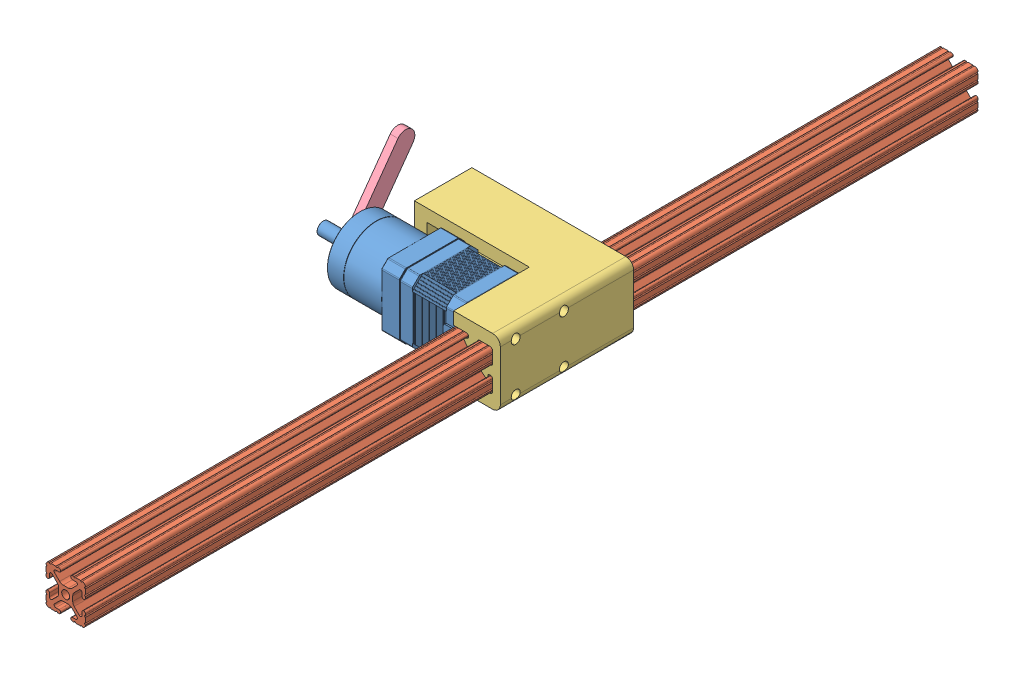
SolidWorks assembly AoA_sub_assm, configuration Default. Lengths in mm.
Overall size (139.5 73.36 574.8).
4 component instances, 4 part files, 7 mates.
Components (placement in the parent):
- 17HS15-1684-HG10-1: 17HS15-1684-HG10 [Default] at (61.1343 21.6253 -23.6268) size (109.65 42.3 53.3)
- 47065T121_T-Slotted Framing-1: 47065T121_T-Slotted Framing [574.8] at (73.2743 21.6253 -23.6268) size (25.4 25.4 574.8)
- Gap AOA Bracket-1: Gap AOA Bracket [Default] at (86.1843 21.6253 -23.6268) x (0 0 -1) z (1 0 0) size (85.81 42.3 104.15)
- GAP_AOA_LeverArm-1: GAP_AOA_LeverArm [Default] at (-26.8157 21.6253 -23.6268) x (0 0.583974 0.811773) z (-1 0 0) size (12 66 5)
Mates (geometry in assembly coordinates):
- Width1: width aligned: plane of Gap AOA Bracket-1 through (85.9743 16.1635 -101.1175) normal (0.038424 0.999262 0); plane of Gap AOA Bracket-1 through (85.9743 27.0871 -101.1175) normal (0.038424 -0.999262 0); plane of 47065T121_T-Slotted Framing-1 through (71.565 17.1295 263.7732) normal (0 -1 0); plane of 47065T121_T-Slotted Framing-1 through (74.9301 26.1211 263.7732) normal (0 1 0)
- Width2: width anti-aligned: plane of Gap AOA Bracket-1 through (76.3028 21.6253 -101.1175) normal (1 0 0); plane of Gap AOA Bracket-1 through (86.1843 21.6253 -23.6268) normal (-1 0 0); plane of 47065T121_T-Slotted Framing-1 through (76.5128 33.2763 263.7732) normal (-1 0 0); plane of 47065T121_T-Slotted Framing-1 through (85.9743 27.9584 263.7732) normal (1 0 0)
- Concentric1: concentric anti-aligned: circle of 17HS15-1684-HG10-1; cylinder of Gap AOA Bracket-1 through (55.7843 37.1253 -8.1268) axis (1 0 0) radius 2
- Concentric2: concentric aligned: circle of 17HS15-1684-HG10-1; circle of Gap AOA Bracket-1
- Width3: width: plane of Gap AOA Bracket-1 through (91.1843 0.4753 1.7732) normal (0 0 1); plane of Gap AOA Bracket-1 through (91.1843 0.4753 -49.0268) normal (0 0 -1); plane of 47065T121_T-Slotted Framing-1 through (66.8579 12.2154 -311.0268) normal (0 0 -1); plane of 47065T121_T-Slotted Framing-1 through (66.8579 12.2154 263.7732) normal (0 0 1)
- Coincident1: coincident anti-aligned: plane of 17HS15-1684-HG10-1 through (-26.8157 21.6253 -23.6268) normal (-1 0 0); plane of GAP_AOA_LeverArm-1 through (-26.8157 21.6253 -23.6268) normal (1 0 0)
- Concentric3: concentric aligned: cylinder of 17HS15-1684-HG10-1 through (-48.3157 21.6253 -23.6268) axis (1 0 0) radius 4; cylinder of GAP_AOA_LeverArm-1 through (-31.8157 21.6253 -23.6268) axis (1 0 0) radius 4
